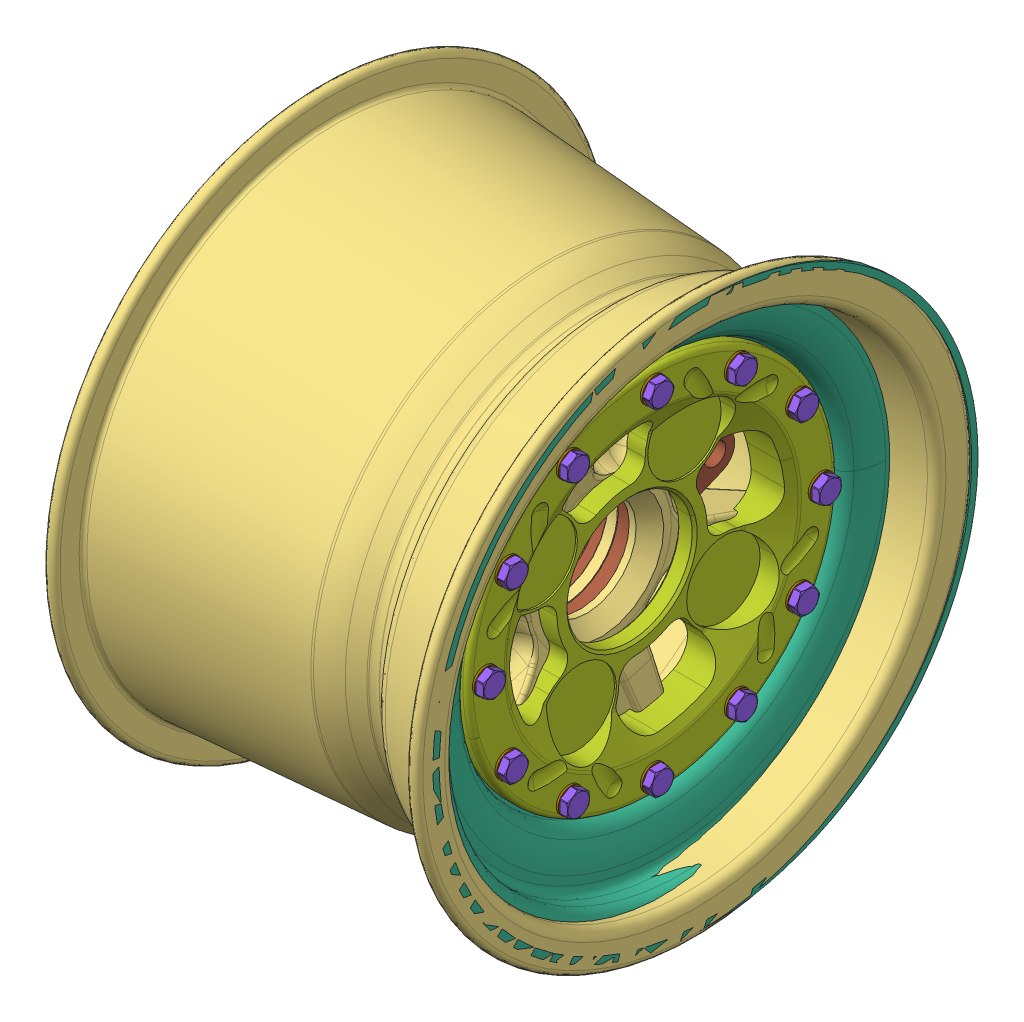
SolidWorks assembly ASSEM_Front_WheelUprBrakes, configuration Default. Lengths in mm.
Overall size (189.81 529.6 398.86).
62 component instances, 13 part files, 21 mates.
Components (placement in the parent):
- Willwood_Calipers-4: Willwood_Calipers [Default] at (-33.147 7.7199 -7.8202) x (0 0.927952 0.372699) z (1 0 0) size (100.77 53.34 71.25)
- 7inRotor_Custom-1: 7inRotor_Custom [Default] at (-30.607 0 0) x (0 -0.991825 -0.127604) z (0 0.127604 -0.991825) size (200.4 5.08 203.2)
- HoosierTyres_43100Slicks-1: HoosierTyres_43100Slicks [Default] at (77.343 0 0) x (0 0.999993 0.00376) z (0 -0.00376 0.999993) size (459.74 205.74 459.74) (hidden)
- OZ 10x7 FSAE wheel.stp-2: OZ 10x7 FSAE wheel.stp [Default] at (-25.6223 0 0) x (0 0.72862 -0.684918) z (1 0 0) size (282.17 282.17 189.8)
- Upright_front-2: Upright_front [Default] at (-51.816 0 0) x (0 0 1) z (-1 0 0) size (169 195.17 25.4)
- UBracket_Upright-1: UBracket_Upright [Default] at (-77.216 83.337 -12.7) x (0 1 0) z (1 0 0) size (31.64 25.4 38.1)
- UBracket_Upright-2: UBracket_Upright [Default] at (-77.216 -86.4314 -14.7215) x (0 1 0) z (1 0 0) size (31.64 25.4 38.1)
- UBracket_Upright-3: UBracket_Upright [Default] at (-77.216 -15.8222 -84.5631) x (0 1 0) z (1 0 0) size (31.64 25.4 38.1)
- Kaiser_10i_4lug-4: Kaiser_10i_4lug [Default] at (31.877 0.0175 -5.138) x (0 0 -1) z (1 0 0) size (276.24 529.6 184.8)
  - 10i 10inch wheel assembly.IGS-1: 10i 10inch wheel assembly.IGS [Default] at origin size (276.24 529.6 184.8)
    - 10in Inner Rim Half_5.in Backspacing [ 10in Inner Rim Half ].IGS-1: 10in Inner Rim Half_5.in Backspacing [ 10in Inner Rim Half ].IGS [Default] at origin size (276.24 388.79 147.39) (hidden)
    - 10in Outer Rim Half.IGS-1: 10in Outer Rim Half.IGS [Default] at origin size (276.24 529.6 37.48)
    - 10-i.IGS-1: 10-i.IGS [Default] at (0 0 10.795) x (0.965926 0.258819 0) z (0 0 1) size (187.34 364.18 19.82)
    - .25 20x1inch hex bolt.2596870A208.IGS-1: .25 20x1inch hex bolt.2596870A208.IGS [Default] at (85.09 0 -0.889) size (12.58 12.7 29.64)
    - .25 20x1inch hex bolt.2596870A208.IGS-2: .25 20x1inch hex bolt.2596870A208.IGS [Default] at (73.6901 42.545 -0.889) x (0.866025 0.5 0) z (0 0 1) size (12.58 12.7 29.64)
    - .25 20x1inch hex bolt.2596870A208.IGS-3: .25 20x1inch hex bolt.2596870A208.IGS [Default] at (42.545 73.6901 -0.889) x (0.5 0.866025 0) z (0 0 1) size (12.58 12.7 29.64)
    - .25 20x1inch hex bolt.2596870A208.IGS-4: .25 20x1inch hex bolt.2596870A208.IGS [Default] at (0 85.09 -0.889) x (0 1 0) z (0 0 1) size (12.58 12.7 29.64)
    - .25 20x1inch hex bolt.2596870A208.IGS-5: .25 20x1inch hex bolt.2596870A208.IGS [Default] at (-42.545 73.6901 -0.889) x (-0.5 0.866025 0) z (0 0 1) size (12.58 12.7 29.64)
    - .25 20x1inch hex bolt.2596870A208.IGS-6: .25 20x1inch hex bolt.2596870A208.IGS [Default] at (-73.6901 42.545 -0.889) x (-0.866025 0.5 0) z (0 0 1) size (12.58 12.7 29.64)
    - .25 20x1inch hex bolt.2596870A208.IGS-7: .25 20x1inch hex bolt.2596870A208.IGS [Default] at (-85.09 0 -0.889) x (-1 0 0) z (0 0 1) size (12.58 12.7 29.64)
    - .25 20x1inch hex bolt.2596870A208.IGS-8: .25 20x1inch hex bolt.2596870A208.IGS [Default] at (-73.6901 -42.545 -0.889) x (-0.866025 -0.5 0) z (0 0 1) size (12.58 12.7 29.64)
    - .25 20x1inch hex bolt.2596870A208.IGS-9: .25 20x1inch hex bolt.2596870A208.IGS [Default] at (-42.545 -73.6901 -0.889) x (-0.5 -0.866025 0) z (0 0 1) size (12.58 12.7 29.64)
    - .25 20x1inch hex bolt.2596870A208.IGS-10: .25 20x1inch hex bolt.2596870A208.IGS [Default] at (0 -85.09 -0.889) x (0 -1 0) z (0 0 1) size (12.58 12.7 29.64)
    - .25 20x1inch hex bolt.2596870A208.IGS-11: .25 20x1inch hex bolt.2596870A208.IGS [Default] at (42.545 -73.6901 -0.889) x (0.5 -0.866025 0) z (0 0 1) size (12.58 12.7 29.64)
    - .25 20x1inch hex bolt.2596870A208.IGS-12: .25 20x1inch hex bolt.2596870A208.IGS [Default] at (73.6901 -42.545 -0.889) x (0.866025 -0.5 0) z (0 0 1) size (12.58 12.7 29.64)
    - washer 94589A300.IGS-1: washer 94589A300.IGS [Default] at (85.09 0 11.811) size (12.71 12.71 1.03)
    - washer 94589A300.IGS-2: washer 94589A300.IGS [Default] at (85.09 0 -3.175) size (12.71 12.71 1.03)
    - washer 94589A300.IGS-3: washer 94589A300.IGS [Default] at (73.6901 42.545 -3.175) x (0.866025 0.5 0) z (0 0 1) size (12.71 12.71 1.03)
    - washer 94589A300.IGS-4: washer 94589A300.IGS [Default] at (42.545 73.6901 -3.175) x (0.5 0.866025 0) z (0 0 1) size (12.71 12.71 1.03)
    - washer 94589A300.IGS-5: washer 94589A300.IGS [Default] at (0 85.09 -3.175) x (0 1 0) z (0 0 1) size (12.71 12.71 1.03)
    - washer 94589A300.IGS-6: washer 94589A300.IGS [Default] at (-42.545 73.6901 -3.175) x (-0.5 0.866025 0) z (0 0 1) size (12.71 12.71 1.03)
    - washer 94589A300.IGS-7: washer 94589A300.IGS [Default] at (-73.6901 42.545 -3.175) x (-0.866025 0.5 0) z (0 0 1) size (12.71 12.71 1.03)
    - washer 94589A300.IGS-8: washer 94589A300.IGS [Default] at (-85.09 0 -3.175) x (-1 0 0) z (0 0 1) size (12.71 12.71 1.03)
    - washer 94589A300.IGS-9: washer 94589A300.IGS [Default] at (-73.6901 -42.545 -3.175) x (-0.866025 -0.5 0) z (0 0 1) size (12.71 12.71 1.03)
    - washer 94589A300.IGS-10: washer 94589A300.IGS [Default] at (-42.545 -73.6901 -3.175) x (-0.5 -0.866025 0) z (0 0 1) size (12.71 12.71 1.03)
    - washer 94589A300.IGS-11: washer 94589A300.IGS [Default] at (0 -85.09 -3.175) x (0 -1 0) z (0 0 1) size (12.71 12.71 1.03)
    - washer 94589A300.IGS-12: washer 94589A300.IGS [Default] at (42.545 -73.6901 -3.175) x (0.5 -0.866025 0) z (0 0 1) size (12.71 12.71 1.03)
    - washer 94589A300.IGS-13: washer 94589A300.IGS [Default] at (73.6901 -42.545 -3.175) x (0.866025 -0.5 0) z (0 0 1) size (12.71 12.71 1.03)
    - washer 94589A300.IGS-14: washer 94589A300.IGS [Default] at (73.6901 42.545 11.811) x (0.866025 0.5 0) z (0 0 1) size (12.71 12.71 1.03)
    - washer 94589A300.IGS-15: washer 94589A300.IGS [Default] at (42.545 73.6901 11.811) x (0.5 0.866025 0) z (0 0 1) size (12.71 12.71 1.03)
    - washer 94589A300.IGS-16: washer 94589A300.IGS [Default] at (0 85.09 11.811) x (0 1 0) z (0 0 1) size (12.71 12.71 1.03)
    - washer 94589A300.IGS-17: washer 94589A300.IGS [Default] at (-42.545 73.6901 11.811) x (-0.5 0.866025 0) z (0 0 1) size (12.71 12.71 1.03)
    - washer 94589A300.IGS-18: washer 94589A300.IGS [Default] at (-73.6901 42.545 11.811) x (-0.866025 0.5 0) z (0 0 1) size (12.71 12.71 1.03)
    - washer 94589A300.IGS-19: washer 94589A300.IGS [Default] at (-85.09 0 11.811) x (-1 0 0) z (0 0 1) size (12.71 12.71 1.03)
    - washer 94589A300.IGS-20: washer 94589A300.IGS [Default] at (-73.6901 -42.545 11.811) x (-0.866025 -0.5 0) z (0 0 1) size (12.71 12.71 1.03)
    - washer 94589A300.IGS-21: washer 94589A300.IGS [Default] at (-42.545 -73.6901 11.811) x (-0.5 -0.866025 0) z (0 0 1) size (12.71 12.71 1.03)
    - washer 94589A300.IGS-22: washer 94589A300.IGS [Default] at (0 -85.09 11.811) x (0 -1 0) z (0 0 1) size (12.71 12.71 1.03)
    - washer 94589A300.IGS-23: washer 94589A300.IGS [Default] at (42.545 -73.6901 11.811) x (0.5 -0.866025 0) z (0 0 1) size (12.71 12.71 1.03)
    - washer 94589A300.IGS-24: washer 94589A300.IGS [Default] at (73.6901 -42.545 11.811) x (0.866025 -0.5 0) z (0 0 1) size (12.71 12.71 1.03)
    - hex nut94804A029.IGS-1: hex nut94804A029.IGS [Default] at (85.09 0 -4.191) size (12.84 12.84 5.78)
    - hex nut94804A029.IGS-2: hex nut94804A029.IGS [Default] at (73.6901 42.545 -4.191) x (0.866025 0.5 0) z (0 0 1) size (12.84 12.84 5.78)
    - hex nut94804A029.IGS-3: hex nut94804A029.IGS [Default] at (42.545 73.6901 -4.191) x (0.5 0.866025 0) z (0 0 1) size (12.84 12.84 5.78)
    - hex nut94804A029.IGS-4: hex nut94804A029.IGS [Default] at (0 85.09 -4.191) x (0 1 0) z (0 0 1) size (12.84 12.84 5.78)
    - hex nut94804A029.IGS-5: hex nut94804A029.IGS [Default] at (-42.545 73.6901 -4.191) x (-0.5 0.866025 0) z (0 0 1) size (12.84 12.84 5.78)
    - hex nut94804A029.IGS-6: hex nut94804A029.IGS [Default] at (-73.6901 42.545 -4.191) x (-0.866025 0.5 0) z (0 0 1) size (12.84 12.84 5.78)
    - hex nut94804A029.IGS-7: hex nut94804A029.IGS [Default] at (-85.09 0 -4.191) x (-1 0 0) z (0 0 1) size (12.84 12.84 5.78)
    - hex nut94804A029.IGS-8: hex nut94804A029.IGS [Default] at (-73.6901 -42.545 -4.191) x (-0.866025 -0.5 0) z (0 0 1) size (12.84 12.84 5.78)
    - hex nut94804A029.IGS-9: hex nut94804A029.IGS [Default] at (-42.545 -73.6901 -4.191) x (-0.5 -0.866025 0) z (0 0 1) size (12.84 12.84 5.78)
    - hex nut94804A029.IGS-10: hex nut94804A029.IGS [Default] at (0 -85.09 -4.191) x (0 -1 0) z (0 0 1) size (12.84 12.84 5.78)
    - hex nut94804A029.IGS-11: hex nut94804A029.IGS [Default] at (42.545 -73.6901 -4.191) x (0.5 -0.866025 0) z (0 0 1) size (12.84 12.84 5.78)
    - hex nut94804A029.IGS-12: hex nut94804A029.IGS [Default] at (73.6901 -42.545 -4.191) x (0.866025 -0.5 0) z (0 0 1) size (12.84 12.84 5.78)
- Spindle-1: Spindle [Default] at (11.43 0 0) x (0 0.141413 -0.989951) z (0 0.989951 0.141413) size (157.22 19.05 157.22)
Mates (geometry in assembly coordinates):
- Concentric1: concentric: circle of assembly; circle of 7inRotor_Custom-1
- Coincident3: coincident: point of Willwood_Calipers-4; circle of assembly
- Distance2: distance = 2.54 mm: plane of assembly through (-33.147 0 0) normal (-1 0 0); plane of assembly; plane of 7inRotor_Custom-1 through (-35.687 0 0) normal (-1 0 0)
- Parallel2: parallel aligned: unknown of Willwood_Calipers-4
- Concentric2: concentric: cylinder of 7inRotor_Custom-1 through (-30.607 0 0) axis (-1 0 0) radius 50; cylinder of HoosierTyres_43100Slicks-1 through (77.343 0 0) axis (1 0 0) radius 152.4
- Concentric3: concentric aligned: cylinder of HoosierTyres_43100Slicks-1 through (77.343 0 0) axis (1 0 0) radius 152.4; circle of OZ 10x7 FSAE wheel.stp-1
- Distance3: distance = 94.869 mm aligned: plane of HoosierTyres_43100Slicks-1 through (-25.527 0 0) normal (1 0 0); plane of OZ 10x7 FSAE wheel.stp-1 through (69.342 0 0) normal (1 0 0)
- Concentric5: concentric: cylinder of 7inRotor_Custom-1 through (-30.607 0 0) axis (-1 0 0) radius 50; cylinder of Upright_front-2 through (-77.216 0 0) axis (1 0 0) radius 38.1
- Coincident11: coincident anti-aligned: plane of Willwood_Calipers-4 through (-58.166 7.7199 -7.8202) normal (1 0 0); plane of Upright_front-2 through (-58.166 0 0) normal (-1 0 0)
- Coincident12: coincident aligned: plane of Upright_front-2 through (-51.816 0 0) normal (0 1 0)
- Concentric6: concentric anti-aligned: cylinder of Willwood_Calipers-4 through (-69.977 8.3618 71.6792) axis (1 0 0) radius 4.064; cylinder of Upright_front-2 through (-51.816 8.3618 71.6792) axis (-1 0 0) radius 4.191
- Coincident15: coincident anti-aligned: plane of Upright_front-2 through (-77.216 0 0) normal (-1 0 0); plane of UBracket_Upright-1 through (-77.216 114.9814 12.7) normal (1 0 0)
- Coincident16: coincident anti-aligned: plane of Upright_front-2 through (-77.216 0 0) normal (-1 0 0); plane of UBracket_Upright-3 through (-77.216 15.8222 -59.1631) normal (1 0 0)
- Coincident17: coincident anti-aligned: plane of Upright_front-2 through (-77.216 0 0) normal (-1 0 0); plane of UBracket_Upright-2 through (-77.216 -54.787 10.6785) normal (1 0 0)
- Coincident18: coincident aligned: cylinder of Upright_front-2 through (-77.216 99.1592 0) axis (1 0 0) radius 6.35; circle of UBracket_Upright-1
- Coincident19: coincident aligned: cylinder of Upright_front-2 through (-77.216 0 -71.8631) axis (1 0 0) radius 6.35; circle of UBracket_Upright-3
- Coincident20: coincident aligned: cylinder of Upright_front-2 through (-77.216 -70.6092 -2.0215) axis (1 0 0) radius 6.35; circle of UBracket_Upright-2
- Tangent2: tangent aligned: plane of OZ 10x7 FSAE wheel.stp-2 through (69.342 0 0) normal (1 0 0); face of ?
- Distance4: distance = 107.95 mm aligned: plane of HoosierTyres_43100Slicks-1 through (77.343 -152.3989 -0.5731) normal (1 0 0); plane of 7inRotor_Custom-1 through (-30.607 0 0) normal (1 0 0)
- Concentric7: concentric: cylinder of 7inRotor_Custom-1 through (-30.607 0 0) axis (-1 0 0) radius 50; cylinder of Spindle-1 through (5.08 0 0) axis (1 0 0) radius 27.94
- Distance5: distance = 5.08 mm anti-aligned: plane of Willwood_Calipers-4 through (0 -24.9394 73.4957) normal (1 0 0); plane of Spindle-1 through (5.08 0 0) normal (-1 0 0)
